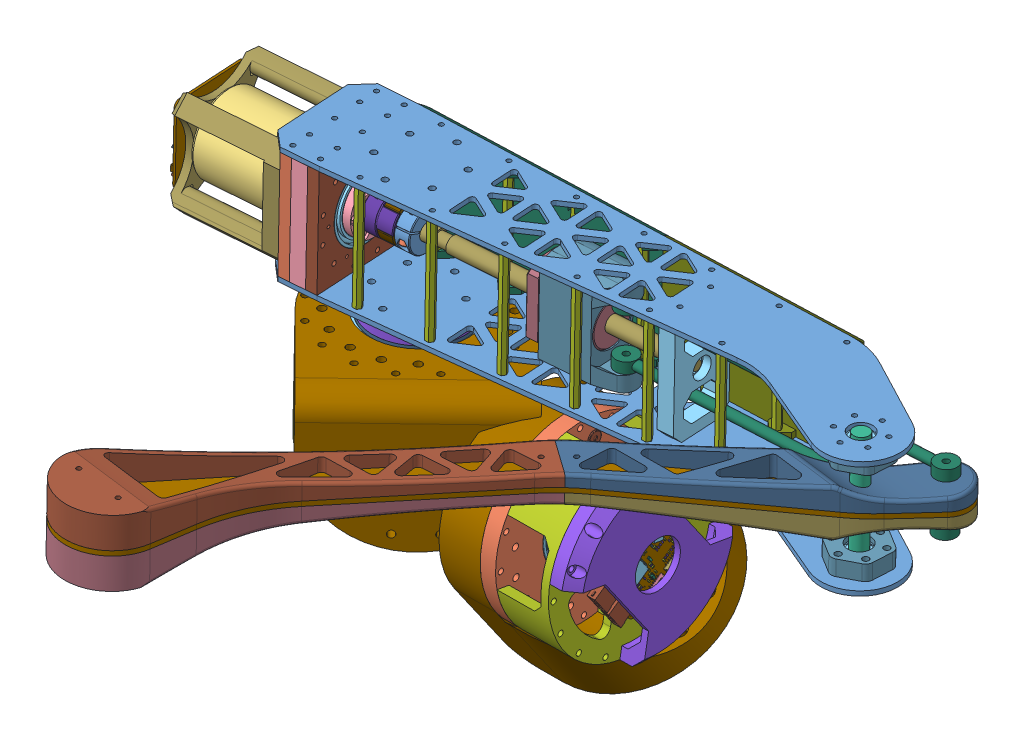
SolidWorks assembly Leg, configuration Default. Lengths in mm. (continued)
Components (placement in the parent): (continued)
- Cycloidal _v3-2: Cycloidal _v3 [Default] at (290.9356 44.932 396.0406) x (-0.007136 -0.180415 -0.983565) z (-0.001309 0.983591 -0.18041) size (173.36 87.57 173.15) (continued)
  - radial ball bearing_68_iso-48: radial ball bearing_68_iso [ISO 15 RBB - 289 - 14,SI,NC,14_68] at (59.3269 82.1622 107.722) x (0.000399 -1 0) z (-0.055662 -0.000022 0.99845) size (5 17 17)
  - m4x14-1: m4x14 [Default] at (47.0925 68.4573 134.6267) x (0.999623 0.000399 0.027466) z (-0.027466 -0.000011 0.999623) size (8 15.2 8)
  - M3x20-1: M3x20 [Default] at (43.4726 96.3558 90.1203) x (-0.837193 -0.000334 -0.546908) z (-0.546908 -0.000218 0.837193) size (6 21.2 6)
  - M3x10-1: M3x10 [Default] at (36.5111 25.853 142.5044) x (0.424034 0.000169 -0.905646) z (0.905646 0.000361 0.424034) size (6 11.2 6)
  - m3x60-1: m3x60 [Default] at (17.1068 35.0453 134.2855) x (-0.837193 -0.000334 -0.546908) z (-0.546908 -0.000218 0.837193) size (5.3 63 5.3)
  - m6-1: m6 [Default] at (60.6129 98.6627 108.4832) x (-0.153131 -0.000061 0.988206) z (0.988206 0.000394 0.153131) size (6 16 6)
Mates (geometry in assembly coordinates):
- Coincident2: coincident anti-aligned: plane of Leg_Upper-1 through (112.6899 202.4857 333.2991) normal (-0.000153 0.999777 -0.0211); plane of Cycloidal_5065-1/Ring_pin_housing_5065-1 through (73.2986 202.5446 336.378) normal (0.000153 -0.999777 0.0211)
- Coincident3: coincident: line of Leg_Upper-1 through (112.6899 202.4857 333.2991) axis (0.996958 -0.001492 -0.077924); plane of Cycloidal_5065-1/Ring_pin_housing_5065-1 through (63.3236 237.5517 336.4187) normal (-0.077938 -0.021048 -0.996736)
- Coincident4: coincident anti-aligned: plane of Cycloidal_5065-1/Ring_pin_housing_5065-1 through (73.2878 272.529 334.901) normal (-0.000153 0.999777 -0.0211); plane of Leg_Upper-2 through (112.6792 272.4701 331.8221) normal (0.000153 -0.999777 0.0211)
- Parallel1: parallel aligned: line of Leg_Upper-1 through (112.6899 202.4857 333.2991) axis (0.996958 -0.001492 -0.077924); line of Leg_Upper-2 through (112.6787 275.4694 331.7588) axis (0.996958 -0.001492 -0.077924)
- Concentric6: concentric anti-aligned: circle of Cycloidal_5065-1/OutPut_shaft_5065-1; cylinder of ball_screw-1 through (275.3766 237.2344 319.8443) axis (-0.996958 0.001492 0.077924) radius 5
- Concentric7: concentric aligned: cylinder of ball_screw-1 through (275.3766 237.2344 319.8443) axis (-0.996958 0.001492 0.077924) radius 5; cylinder of ball_screw_slider-1 through (230.2255 237.302 323.3734) axis (-0.996958 0.001492 0.077924) radius 5
- Concentric8: concentric aligned: cylinder of ball_screw_slider-1 through (230.2255 237.302 323.3734) axis (-0.996958 0.001492 0.077924) radius 14; cylinder of connection_rod_base-1 through (230.2255 237.302 323.3734) axis (-0.996958 0.001492 0.077924) radius 14
- Coincident10: coincident anti-aligned: plane of ball_screw_slider-1 through (198.3229 237.3497 325.867) normal (0.996958 -0.001492 -0.077924); plane of connection_rod_base-1 through (198.3229 237.3497 325.867) normal (-0.996958 0.001492 0.077924)
- Concentric9: concentric aligned: cylinder of Link_Rod-1 through (438.9166 257.092 311.7001) axis (0.000153 -0.999777 0.0211) radius 7; cylinder of Link_Rod-2 through (438.9216 224.0994 312.3964) axis (0.000153 -0.999777 0.0211) radius 7
- Concentric10: concentric aligned: circle of connection_rod_base-1; circle of Link_Rod-1
- Concentric11: concentric anti-aligned: cylinder of connection_rod_base-1 through (239.2073 177.3019 323.9381) axis (-0.000153 0.999777 -0.0211) radius 2.5; cylinder of Link_Rod-2 through (239.2002 224.2914 322.9464) axis (0.000153 -0.999777 0.0211) radius 2
- Coincident11: coincident anti-aligned: plane of connection_rod_base-1 through (230.2225 257.2975 322.9514) normal (0.000153 -0.999777 0.0211); circle of Link_Rod-1
- Coincident12: coincident anti-aligned: plane of connection_rod_base-1 through (230.2286 217.3064 323.7954) normal (-0.000153 0.999777 -0.0211); plane of Link_Rod-2 through (239.2012 217.293 323.0941) normal (0.000153 -0.999777 0.0211)
- Parallel2: parallel aligned: plane of ball_screw_slider-1 through (189.1781 237.0459 311.5393) normal (-0.077938 -0.021048 -0.996736); plane of connection_rod_base-1 through (229.0565 236.9863 308.4224) normal (-0.077938 -0.021048 -0.996736)
- Concentric13: concentric anti-aligned: cylinder of ball_screw-1 through (104.8968 237.4895 333.1693) axis (0.996958 -0.001492 -0.077924) radius 4; cylinder of Shaft Coupler D25L30 8x8.step-1/8x8_Flexible_Spider_Shaft_Coupling.step-1/Coupler L.step-1 through (111.8755 237.4791 332.6238) axis (-0.996958 0.001492 0.077924) radius 4
- Coincident14: coincident anti-aligned: plane of ball_screw-1 through (116.8603 237.4716 332.2342) normal (-0.996958 0.001492 0.077924); plane of Shaft Coupler D25L30 8x8.step-1/8x8_Flexible_Spider_Shaft_Coupling.step-1/Coupler L.step-1 through (116.8603 237.4716 332.2342) normal (0.996958 -0.001492 -0.077924)
- Concentric14: concentric anti-aligned: cylinder of Shaft Coupler D25L30 8x8.step-1/8x8_Flexible_Spider_Shaft_Coupling.step-1/Coupler R.step-1 through (86.951 237.5191 334.5651) axis (0.996958 -0.001492 -0.077924) radius 4; cylinder of m8-1 through (98.9145 237.5012 333.63) axis (-0.996958 0.001492 0.077924) radius 4
- Coincident15: coincident anti-aligned: plane of Shaft Coupler D25L30 8x8.step-1/8x8_Flexible_Spider_Shaft_Coupling.step-1/Coupler R.step-1 through (86.951 237.5191 334.5651) normal (-0.996958 0.001492 0.077924); plane of m8-1 through (86.951 237.5191 334.5651) normal (0.996958 -0.001492 -0.077924)
- Concentric15: concentric aligned: cylinder of Cycloidal_5065-1/OutPut_shaft_5065-1 through (80.2719 237.5264 335.094) axis (-0.996958 0.001492 0.077924) radius 9; cylinder of Output_Shaft_holder-1 through (85.2567 237.5189 334.7044) axis (-0.996958 0.001492 0.077924) radius 17.5
- Concentric16: concentric aligned: cylinder of Cycloidal_5065-1/OutPut_shaft_5065-1 through (79.7382 249.604 328.0338) axis (-0.996958 0.001492 0.077924) radius 1.5; cylinder of Output_Shaft_holder-1 through (84.7229 249.5965 327.6442) axis (-0.996958 0.001492 0.077924) radius 1.5
- Coincident17: coincident aligned: plane of m8-1 through (80.2714 237.5291 335.0872) normal (-0.996958 0.001492 0.077924); plane of Output_Shaft_holder-1 through (80.2719 237.5264 335.094) normal (-0.996958 0.001492 0.077924)
- Coincident18: coincident anti-aligned: plane of Cycloidal_5065-1/OutPut_shaft_5065-1 through (80.2719 237.5264 335.094) normal (0.996958 -0.001492 -0.077924); plane of Output_Shaft_holder-1 through (80.2719 237.5264 335.094) normal (-0.996958 0.001492 0.077924)
- Concentric17: concentric anti-aligned: cylinder of ball_screw-1 through (282.3553 237.224 319.2988) axis (-0.996958 0.001492 0.077924) radius 3; cylinder of ball_screw_holder-1 through (275.3766 237.2344 319.8443) axis (0.996958 -0.001492 -0.077924) radius 6.5
- Coincident22: coincident aligned: plane of Leg_Upper-1 through (112.6903 199.4863 333.3624) normal (0.000153 -0.999777 0.0211); plane of m10-1 through (412.5361 199.7352 342.9773) normal (0.000153 -0.999777 0.0211)
- Concentric20: concentric anti-aligned: cylinder of Leg_Upper-1 through (412.5357 202.7345 342.914) axis (0.000153 -0.999777 0.0211) radius 7.5; cylinder of radial ball bearing_68_iso-3 through (412.5384 185.1009 343.2861) axis (-0.000153 0.999777 -0.0211) radius 11
- Concentric21: concentric anti-aligned: cylinder of m10-1 through (412.5245 275.7182 341.3737) axis (0.000153 -0.999777 0.0211) radius 5; cylinder of radial ball bearing_68_iso-4 through (412.5286 249.0867 341.9357) axis (-0.000153 0.999777 -0.0211) radius 5
- Coincident27: coincident anti-aligned: plane of Cycloidal_5065-1/Ring_pin_housing_5065-1 through (73.2878 272.529 334.901) normal (-0.000153 0.999777 -0.0211); plane of Leg_Upper-2 through (112.6792 272.4701 331.8221) normal (0.000153 -0.999777 0.0211)
- Coincident28: coincident anti-aligned: plane of Leg_Upper-1 through (112.6899 202.4857 333.2991) normal (-0.000153 0.999777 -0.0211); plane of Cycloidal_5065-1/Ring_pin_housing_5065-1 through (73.2986 202.5446 336.378) normal (0.000153 -0.999777 0.0211)
- Coincident29: coincident aligned: plane of Cycloidal_5065-1/Motor_cover_5065-1 through (46.3677 287.566 336.6884) normal (-0.996958 0.001492 0.077924); plane of Leg_Upper-2 through (46.3695 275.5686 336.9416) normal (-0.996958 0.001492 0.077924)
- Concentric23: concentric anti-aligned: cylinder of Leg_Upper-2 through (412.5245 275.7182 341.3737) axis (0.000153 -0.999777 0.0211) radius 7.5; cylinder of radial ball bearing_68_iso-4 through (412.5286 249.0867 341.9357) axis (-0.000153 0.999777 -0.0211) radius 11
- Coincident32: coincident anti-aligned: plane of Leg_Upper-1 through (112.6899 202.4857 333.2991) normal (-0.000153 0.999777 -0.0211); plane of brass_spacer_70mm-6 through (355.7642 201.728 295.6372) normal (0.000153 -0.999777 0.0211)
- Coincident33: coincident anti-aligned: plane of Leg_Upper-1 through (112.6899 202.4857 333.2991) normal (-0.000153 0.999777 -0.0211); plane of brass_spacer_70mm-7 through (312.7935 201.755 297.2247) normal (0.000153 -0.999777 0.0211)
- Coincident34: coincident anti-aligned: plane of Leg_Upper-1 through (112.6899 202.4857 333.2991) normal (-0.000153 0.999777 -0.0211); plane of brass_spacer_70mm-1 through (140.9108 201.8627 303.5749) normal (0.000153 -0.999777 0.0211)
- Coincident35: coincident anti-aligned: plane of Leg_Upper-1 through (112.6899 202.4857 333.2991) normal (-0.000153 0.999777 -0.0211); plane of brass_spacer_70mm-2 through (97.9401 201.8896 305.1625) normal (0.000153 -0.999777 0.0211)
- Coincident36: coincident anti-aligned: plane of Leg_Upper-1 through (112.6899 202.4857 333.2991) normal (-0.000153 0.999777 -0.0211); plane of brass_spacer_70mm-3 through (269.8228 201.7819 298.8123) normal (0.000153 -0.999777 0.0211)
- Coincident37: coincident anti-aligned: plane of Leg_Upper-1 through (112.6899 202.4857 333.2991) normal (-0.000153 0.999777 -0.0211); plane of brass_spacer_70mm-4 through (226.8521 201.8088 300.3998) normal (0.000153 -0.999777 0.0211)
- Coincident38: coincident anti-aligned: plane of Leg_Upper-1 through (112.6899 202.4857 333.2991) normal (-0.000153 0.999777 -0.0211); plane of brass_spacer_70mm-5 through (183.8815 201.8357 301.9874) normal (0.000153 -0.999777 0.0211)
- Concentric24: concentric anti-aligned: cylinder of Leg_Upper-1 through (97.9416 191.8918 305.3735) axis (-0.000153 0.999777 -0.0211) radius 1.5; cylinder of brass_spacer_70mm-2 through (97.9294 271.874 303.6855) axis (0.000153 -0.999777 0.0211) radius 1.5
- Coincident39: coincident aligned: cylinder of Leg_Upper-1 through (140.9123 191.8649 303.7859) axis (-0.000153 0.999777 -0.0211) radius 1.5; circle of brass_spacer_70mm-1
- Coincident40: coincident aligned: cylinder of Leg_Upper-1 through (183.883 191.838 302.1984) axis (-0.000153 0.999777 -0.0211) radius 1.5; circle of brass_spacer_70mm-5
- Concentric25: concentric anti-aligned: cylinder of Leg_Upper-1 through (226.8537 191.811 300.6108) axis (-0.000153 0.999777 -0.0211) radius 1.5; cylinder of brass_spacer_70mm-4 through (226.8414 271.7932 298.9228) axis (0.000153 -0.999777 0.0211) radius 1.5
- Coincident41: coincident anti-aligned: circle of Leg_Upper-1; cylinder of brass_spacer_70mm-3 through (269.8121 271.7663 297.3353) axis (0.000153 -0.999777 0.0211) radius 1.5
- Concentric26: concentric anti-aligned: cylinder of Leg_Upper-1 through (312.795 191.7572 297.4357) axis (-0.000153 0.999777 -0.0211) radius 1.5; cylinder of brass_spacer_70mm-7 through (312.7828 271.7394 295.7478) axis (0.000153 -0.999777 0.0211) radius 1.5
- Concentric27: concentric anti-aligned: cylinder of Leg_Upper-1 through (355.7657 191.7303 295.8482) axis (-0.000153 0.999777 -0.0211) radius 1.5; cylinder of brass_spacer_70mm-6 through (355.7535 271.7125 294.1602) axis (0.000153 -0.999777 0.0211) radius 1.5
- Coincident42: coincident anti-aligned: plane of Leg_Upper-2 through (112.6792 272.4701 331.8221) normal (0.000153 -0.999777 0.0211); plane of brass_spacer_70mm-9 through (230.5948 272.8042 346.7992) normal (-0.000153 0.999777 -0.0211)
- Coincident43: coincident anti-aligned: plane of Leg_Upper-2 through (112.6792 272.4701 331.8221) normal (0.000153 -0.999777 0.0211); plane of brass_spacer_70mm-8 through (273.2998 272.7047 341.7715) normal (-0.000153 0.999777 -0.0211)
- Coincident44: coincident anti-aligned: plane of Leg_Upper-2 through (112.6792 272.4701 331.8221) normal (0.000153 -0.999777 0.0211); plane of brass_spacer_70mm-10 through (316.0047 272.6051 336.7437) normal (-0.000153 0.999777 -0.0211)
- Concentric28: concentric anti-aligned: cylinder of Leg_Upper-2 through (316.0058 265.6066 336.8914) axis (-0.000153 0.999777 -0.0211) radius 1.5; cylinder of brass_spacer_70mm-10 through (316.0047 272.6051 336.7437) axis (0.000153 -0.999777 0.0211) radius 1.5
- Coincident45: coincident anti-aligned: axis of Leg_Upper-2 through (273.2998 272.7047 341.7715) axis (-0.000153 0.999777 -0.0211); line of brass_spacer_70mm-8 through (273.2998 272.7047 341.7715) axis (0.000153 -0.999777 0.0211)
- Concentric29: concentric anti-aligned: cylinder of Leg_Upper-2 through (230.5959 265.8058 346.9469) axis (-0.000153 0.999777 -0.0211) radius 1.5; cylinder of brass_spacer_70mm-9 through (230.5948 272.8042 346.7992) axis (0.000153 -0.999777 0.0211) radius 1.5
- Coincident46: coincident anti-aligned: circle of Leg_Upper-2; cylinder of brass_spacer_70mm-12 through (102.48 273.1029 361.8825) axis (0.000153 -0.999777 0.0211) radius 1.5
- Coincident47: coincident anti-aligned: circle of Leg_Upper-2; cylinder of brass_spacer_70mm-11 through (187.8899 272.9038 351.827) axis (0.000153 -0.999777 0.0211) radius 1.5
- Concentric31: concentric anti-aligned: cylinder of brass_spacer_70mm-13 through (145.1849 273.0034 356.8547) axis (0.000153 -0.999777 0.0211) radius 1.5; cylinder of Leg_Upper-2 through (145.186 266.0049 357.0024) axis (-0.000153 0.999777 -0.0211) radius 1.5
- Coincident48: coincident: plane of Leg_Upper-2 through (112.6792 272.4701 331.8221) normal (0.000153 -0.999777 0.0211); line of brass_spacer_70mm-11 through (190.5457 272.9042 351.827) axis (-0.499999 -0.01835 -0.865832)
- Coincident49: coincident anti-aligned: plane of Leg_Upper-2 through (112.6792 272.4701 331.8221) normal (0.000153 -0.999777 0.0211); circle of brass_spacer_70mm-13
- Coincident50: coincident anti-aligned: plane of Leg_Upper-2 through (112.6792 272.4701 331.8221) normal (0.000153 -0.999777 0.0211); plane of brass_spacer_70mm-12 through (102.48 273.1029 361.8825) normal (-0.000153 0.999777 -0.0211)
- Coincident51: coincident anti-aligned: plane of Leg_Upper-1 through (112.6903 199.4863 333.3624) normal (0.000153 -0.999777 0.0211); plane of Output_2-1 through (112.6893 199.4863 333.3623) normal (-0.000153 0.999777 -0.0211)
- Concentric32: concentric aligned: line of Leg_Upper-1 through (111.9525 202.9706 356.2821) axis (0.000153 -0.999777 0.0211); cylinder of Output_2-1 through (111.953 199.9713 356.3454) axis (0.000153 -0.999777 0.0211) radius 2.1
- Concentric33: concentric aligned: cylinder of Leg_Upper-1 through (113.4273 202.0007 310.316) axis (0.000153 -0.999777 0.0211) radius 2; line of Output_2-1 through (113.4277 199.0014 310.3793) axis (0.000153 -0.999777 0.0211)
- Concentric39: concentric anti-aligned: cylinder of m10-1 through (412.5245 275.7182 341.3737) axis (0.000153 -0.999777 0.0211) radius 5; cylinder of radial ball bearing_68_iso-3 through (412.5384 185.1009 343.2861) axis (-0.000153 0.999777 -0.0211) radius 5
- Coincident59: coincident anti-aligned: plane of Leg_Upper-2 through (112.6792 272.4701 331.8221) normal (0.000153 -0.999777 0.0211); plane of ball_screw_holder-1 through (276.93 272.6476 339.0405) normal (-0.000153 0.999777 -0.0211)
- LimitDistance1: limit distance = 65.7111 mm anti-aligned: plane of ball_screw_slider-1 through (190.3472 237.3617 326.4903) normal (-0.996958 0.001492 0.077924); plane of ball_screw-1 through (124.8359 237.4597 331.6108) normal (0.996958 -0.001492 -0.077924)
- Concentric42: concentric aligned: cylinder of m10-1 through (412.5245 275.7182 341.3737) axis (0.000153 -0.999777 0.0211) radius 5; cylinder of Leg_Lower-1/Leg_Lower_out_left_1-1 through (412.527 259.2219 341.7218) axis (0.000153 -0.999777 0.0211) radius 5
- Concentric43: concentric anti-aligned: circle of Link_Rod-1; cylinder of Leg_Lower-1/Leg_Lower_out_left_1-1 through (438.9163 258.5917 311.6684) axis (0.000153 -0.999777 0.0211) radius 2
- Coincident62: coincident aligned: plane of Cycloidal_5065-1/Ring_pin_housing_5065-1 through (63.3236 237.5517 336.4187) normal (-0.000153 0.999777 -0.0211); plane of Leg_Lower-1/Leg_Lower_in-1 through (412.5303 237.7267 342.1755) normal (-0.000153 0.999777 -0.0211)
- Concentric45: concentric anti-aligned: cylinder of radial ball bearing_68_iso-3 through (412.5384 185.1009 343.2861) axis (-0.000153 0.999777 -0.0211) radius 11; cylinder of bearing_knee_holder-2 through (412.5341 212.7323 342.703) axis (0.000153 -0.999777 0.0211) radius 11
- Coincident65: coincident aligned: plane of radial ball bearing_68_iso-3 through (404.3203 202.6459 338.774) normal (0.000153 -0.999777 0.0211); plane of bearing_knee_holder-2 through (401.7449 202.5915 336.2152) normal (0.000153 -0.999777 0.0211)
- Coincident69: coincident anti-aligned: plane of Leg_Upper-1 through (112.6899 202.4857 333.2991) normal (-0.000153 0.999777 -0.0211); plane of bearing_knee_holder-2 through (401.7449 202.5915 336.2152) normal (0.000153 -0.999777 0.0211)
- Concentric46: concentric aligned: cylinder of radial ball bearing_68_iso-4 through (412.5286 249.0867 341.9357) axis (-0.000153 0.999777 -0.0211) radius 11; cylinder of bearing_knee_holder-3 through (412.5265 262.7211 341.648) axis (-0.000153 0.999777 -0.0211) radius 11
- Coincident70: coincident anti-aligned: plane of Leg_Upper-2 through (112.6792 272.4701 331.8221) normal (0.000153 -0.999777 0.0211); plane of bearing_knee_holder-3 through (412.9322 272.4511 328.7446) normal (-0.000153 0.999777 -0.0211)
- Coincident71: coincident aligned: plane of bearing_knee_holder-2 through (414.4868 213.0934 359.8024) normal (0.471978 0.018674 0.881412); plane of bearing_knee_holder-3 through (425.6771 262.9575 352.7537) normal (0.471978 0.018674 0.881412)
- Parallel5: parallel aligned: plane of bearing_knee_holder-2 through (428.3223 212.8794 349.5619) normal (0.999486 0.000829 0.03205); plane of bearing_knee_holder-3 through (428.7219 262.6005 335.8146) normal (0.999486 0.000829 0.03205)
- Concentric47: concentric anti-aligned: cylinder of Leg_Upper-1 through (400.6355 192.8693 349.4953) axis (-0.000153 0.999777 -0.0211) radius 1.5; cylinder of bearing_knee_holder-2 through (400.6324 212.8649 349.0733) axis (0.000153 -0.999777 0.0211) radius 2
- Concentric48: concentric anti-aligned: cylinder of ball_screw-1 through (282.3553 237.224 319.2988) axis (-0.996958 0.001492 0.077924) radius 3; cylinder of radial ball bearing_68_iso-1 through (257.2943 237.2615 321.2577) axis (0.996958 -0.001492 -0.077924) radius 3
- Coincident73: coincident aligned: plane of ball_screw-1 through (275.3766 237.2344 319.8443) normal (0.996958 -0.001492 -0.077924); circle of radial ball bearing_68_iso-1
- Coincident74: coincident anti-aligned: plane of ball_screw_holder-1 through (275.3766 237.2344 319.8443) normal (-0.996958 0.001492 0.077924); circle of radial ball bearing_68_iso-1
- Coincident75: coincident anti-aligned: plane of Leg_Upper-2 through (112.6792 272.4701 331.8221) normal (0.000153 -0.999777 0.0211); circle of radial ball bearing_68_iso-4
- Coincident76: coincident anti-aligned: plane of Leg_Upper-2 through (111.4407 274.7594 298.127) normal (-0.036778 -0.021091 -0.999101); plane of leg_cover-1 through (77.7616 271.7811 299.4296) normal (0.036778 0.021091 0.999101)
- Coincident77: coincident aligned: line of Leg_Upper-2 through (77.5358 274.7806 299.3746) axis (0.999323 -0.000623 -0.036773); line of leg_cover-1 through (77.7612 274.7804 299.3663) axis (0.999323 -0.000623 -0.036773)
- Parallel6: parallel: plane of brass_spacer_70mm-4 through (228.253 271.8409 301.1719) normal (0.883828 0.010006 0.467704); line of leg_cover-1 through (228.8781 267.8176 300.106) axis (0.467811 -0.018577 -0.883633)
- Parallel7: parallel anti-aligned: plane of brass_spacer_70mm-1 through (143.5541 271.8454 302.0003) normal (0.847051 -0.011085 -0.531397); plane of leg_cover-1 through (176.8365 199.9857 356.5577) normal (-0.847051 0.011085 0.531397)
- Coincident79: coincident anti-aligned: plane of Leg_Upper-1 through (111.4519 201.7757 299.6672) normal (-0.036778 -0.021091 -0.999101); plane of leg_cover_2-1 through (234.1558 271.6836 293.6746) normal (0.036778 0.021091 0.999101)
- Coincident80: coincident anti-aligned: plane of leg_cover-1 through (234.1651 210.9123 294.9572) normal (0.999323 -0.000623 -0.036773); plane of leg_cover_2-1 through (234.1651 210.9123 294.9572) normal (-0.999323 0.000623 0.036773)
- Coincident81: coincident aligned: line of Leg_Upper-2 through (77.5358 274.7806 299.3746) axis (0.999323 -0.000623 -0.036773); line of leg_cover_2-1 through (234.1553 274.6829 293.6113) axis (0.999323 -0.000623 -0.036773)
- Coincident85: coincident anti-aligned: plane of brass_spacer_70mm-2 through (100.5834 271.8724 303.5878) normal (0.847051 -0.011085 -0.531397); plane of leg_cover-1 through (133.8656 200.0125 358.1389) normal (-0.847051 0.011085 0.531397)
- Parallel9: parallel anti-aligned: plane of brass_spacer_70mm-5 through (186.5248 271.8185 300.4127) normal (0.847051 -0.011085 -0.531397); plane of leg_cover-1 through (219.8074 199.9589 354.9764) normal (-0.847051 0.011085 0.531397)
- Parallel10: parallel anti-aligned: plane of brass_spacer_70mm-3 through (272.4661 271.7647 297.2376) normal (0.847051 -0.011085 -0.531397); plane of leg_cover_2-1 through (294.3217 199.5193 333.6065) normal (-0.847051 0.011085 0.531397)
- Parallel11: parallel aligned: plane of brass_spacer_70mm-7 through (311.3712 271.6917 293.4987) normal (-0.883828 -0.010006 -0.467704); plane of leg_cover_2-1 through (338.7264 197.8305 253.2634) normal (-0.883828 -0.010006 -0.467704)
- Parallel12: parallel anti-aligned: plane of brass_spacer_70mm-6 through (358.4075 271.7108 294.0625) normal (0.847051 -0.011085 -0.531397); plane of leg_cover_2-1 through (380.2635 199.4657 330.444) normal (-0.847051 0.011085 0.531397)
- Coincident86: coincident anti-aligned: plane of Output_2-1 through (112.6906 191.4881 333.5311) normal (0.000153 -0.999777 0.0211); plane of Cycloidal_v3-1/Output_Shaft-1 through (113.1603 181.6466 333.5603) normal (-0.00015 0.999786 -0.020701)
- Concentric49: concentric aligned: cylinder of Output_2-1 through (112.6893 199.4863 333.3623) axis (0.000153 -0.999777 0.0211) radius 30; cylinder of Cycloidal _v3-1/Cover_new-1 through (112.6906 191.4881 333.5311) axis (0.000153 -0.999777 0.0211) radius 57.5
- Coincident90: coincident anti-aligned: plane of Output_2-2 through (193.6649 124.5302 333.9109) normal (0.999971 -0.000072 -0.007648); plane of Cycloidal_v3-2/Output_Shaft-1 through (193.6668 124.0999 334.1678) normal (-0.999974 0 0.007256)
- Concentric53: concentric aligned: cylinder of Output_2-2 through (185.6651 124.5307 333.972) axis (0.999971 -0.000072 -0.007648) radius 30; cylinder of Cycloidal _v3-2/Cover_new-1 through (183.8252 124.5309 333.9861) axis (0.999971 -0.000072 -0.007648) radius 57.5
- Coincident91: coincident anti-aligned: plane of Output_2-1 through (112.6906 191.4881 333.5311) normal (0.000153 -0.999777 0.0211); plane of Cycloidal _v3-1/Output_Shaft-2 through (112.6906 191.4881 333.5311) normal (-0.000153 0.999777 -0.0211)
